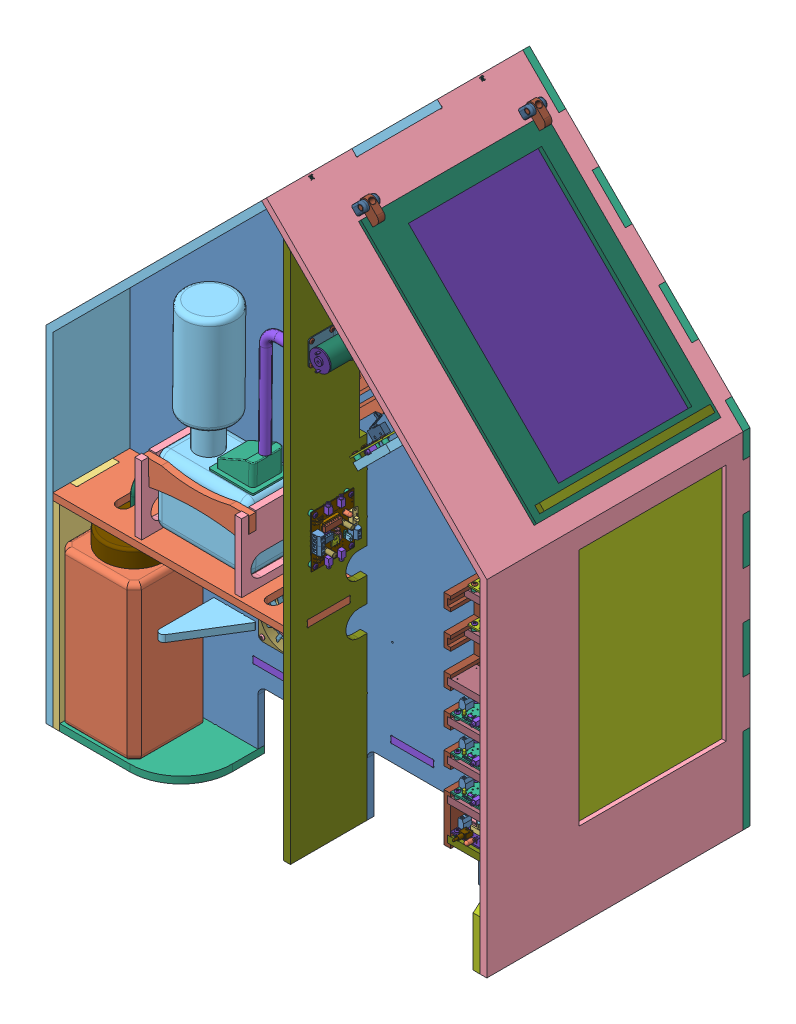
SolidWorks assembly Serre Toutes Options, configuration OLED. Lengths in mm. (continued)
Mates (geometry in assembly coordinates): (continued)
- Coïncidente51: coincident aligned: plane of FONDINTERIEUR-1 through (-297.9367 -225.0262 -4) normal (0 0 -1); plane of VIS TORCX TF 3 X 19-3 through (-31.2492 -313.1905 -4) normal (0 0 -1)
- Coïncidente52: coincident anti-aligned: axis of FONDINTERIEUR-1 through (-30.876 -274.5499 -4) axis (0 0 1); axis of VIS TORCX TF 3 X 19-4 through (-30.876 -274.5499 12.4885) axis (0 0 -1)
- Coïncidente53: coincident aligned: plane of FONDINTERIEUR-1 through (-297.9367 -225.0262 -4) normal (0 0 -1); plane of VIS TORCX TF 3 X 19-4 through (-31.2492 -271.7749 -4) normal (0 0 -1)
- Coïncidente54: coincident anti-aligned: axis of FONDINTERIEUR-1 through (-169.876 -89.9656 -4) axis (0 0 1); axis of VIS TORCX TF 3 X 19-5 through (-169.876 -89.9656 12.4885) axis (0 0 -1)
- Coïncidente55: coincident aligned: plane of FONDINTERIEUR-1 through (-297.9367 -225.0262 -4) normal (0 0 -1); plane of VIS TORCX TF 3 X 19-5 through (-170.2492 -87.1905 -4) normal (0 0 -1)
- Coïncidente56: coincident anti-aligned: axis of FONDINTERIEUR-1 through (-30.876 -27.0369 -4) axis (0 0 1); axis of VIS TORCX TF 3 X 19-6 through (-30.876 -27.0369 12.4885) axis (0 0 -1)
- Coïncidente57: coincident aligned: plane of FONDINTERIEUR-1 through (-297.9367 -225.0262 -4) normal (0 0 -1); plane of VIS TORCX TF 3 X 19-6 through (-31.2492 -24.2619 -4) normal (0 0 -1)
- Coïncidente58: coincident anti-aligned: axis of FONDINTERIEUR-1 through (-30.876 278.5344 -4) axis (0 0 1); axis of VIS TORCX TF 3 X 19-7 through (-30.876 278.5344 12.4885) axis (0 0 -1)
- Coïncidente59: coincident aligned: plane of FONDINTERIEUR-1 through (-297.9367 -225.0262 -4) normal (0 0 -1); plane of VIS TORCX TF 3 X 19-7 through (-31.2492 281.3095 -4) normal (0 0 -1)
- Coïncidente60: coincident anti-aligned: plane of FONDINTERIEUR-1 through (-296.876 -226.0869 4) normal (-1 0 0); plane of Coté gauche serre-1 through (-296.876 -275.0426 -2.9402) normal (1 0 0)
- Coïncidente61: coincident anti-aligned: plane of FONDINTERIEUR-1 through (-298.9973 -273.9656 4) normal (0 1 0); plane of Coté gauche serre-1 through (-296.876 -273.9656 1.8944) normal (0 -1 0)
- Coïncidente62: coincident anti-aligned: plane of FONDINTERIEUR-1 through (-297.9367 -225.0262 -4) normal (0 0 -1); plane of Coté gauche serre-1 through (-296.876 -323.9656 -4) normal (0 0 1)
- Coïncidente63: coincident anti-aligned: plane of FONDINTERIEUR-1 through (-154.876 -315.9656 -4) normal (0 -1 0); plane of suportbloceau-1 through (-297.9367 -315.9656 75.0607) normal (0 1 0)
- Coïncidente64: coincident anti-aligned: plane of FONDINTERIEUR-1 through (-204.876 -318.0869 -4) normal (1 0 0); plane of suportbloceau-1 through (-204.876 -315.9656 -4) normal (-1 0 0)
- Coïncidente65: coincident aligned: plane of FONDINTERIEUR-1 through (-297.9367 -225.0262 -4) normal (0 0 -1); plane of suportbloceau-1 through (-154.876 -315.9656 -4) normal (0 0 -1)
- Coïncidente66: coincident anti-aligned: plane of FONDINTERIEUR-1 through (-95.876 -28.0869 4) normal (1 0 0); plane of Coté support brumisateur-1 through (-95.876 -24.9049 2.9393) normal (-1 0 0)
- Coïncidente67: coincident anti-aligned: plane of FONDINTERIEUR-1 through (-89.9973 -65.9656 4) normal (0 1 0); plane of Coté support brumisateur-1 through (-95.876 -65.9656 -4) normal (0 -1 0)
- Coïncidente68: coincident aligned: plane of FONDINTERIEUR-1 through (-297.9367 -225.0262 -4) normal (0 0 -1); plane of Coté support brumisateur-1 through (-95.876 -25.9656 -4) normal (0 0 -1)
- Coïncidente69: coincident anti-aligned: plane of FONDINTERIEUR-1 through (-212.876 -28.0869 4) normal (1 0 0); plane of Coté support brumisateur-2 through (-212.876 -24.9049 2.9393) normal (-1 0 0)
- Coïncidente70: coincident anti-aligned: plane of FONDINTERIEUR-1 through (-210.7547 -65.9656 4) normal (0 1 0); plane of Coté support brumisateur-2 through (-212.876 -65.9656 -4) normal (0 -1 0)
- Coïncidente71: coincident aligned: plane of FONDINTERIEUR-1 through (-297.9367 -225.0262 -4) normal (0 0 -1); plane of Coté support brumisateur-2 through (-212.876 -25.9656 -4) normal (0 0 -1)
- Coïncidente72: coincident anti-aligned: plane of FONDINTERIEUR-1 through (-189.2547 -195.9656 -4) normal (0 1 0); plane of Renfort bidon-1 through (-192.4367 -195.9656 2.9393) normal (0 -1 0)
- Coïncidente73: coincident anti-aligned: plane of FONDINTERIEUR-1 through (-191.376 -190.0869 -4) normal (1 0 0); plane of Renfort bidon-1 through (-191.376 -187.9656 1.8787) normal (-1 0 0)
- Coïncidente74: coincident aligned: plane of FONDINTERIEUR-1 through (-297.9367 -225.0262 -4) normal (0 0 -1); plane of Renfort bidon-1 through (-191.376 -187.9656 -4) normal (0 0 -1)
- Coïncidente75: coincident aligned: axis of FONDINTERIEUR-1 through (-198.876 -191.9656 4) axis (0 0 -1); axis of VIS TORCX TF 3 X 19-12 through (-198.876 -191.9656 12.4885) axis (0 0 -1)
- Coïncidente76: coincident aligned: plane of FONDINTERIEUR-1 through (-297.9367 -225.0262 -4) normal (0 0 -1); plane of VIS TORCX TF 3 X 19-12 through (-199.9485 -189.3791 -4) normal (0 0 -1)
- Coïncidente77: coincident aligned: axis of FONDINTERIEUR-1 through (-164.4919 -191.9656 4) axis (0 0 -1); axis of VIS TORCX TF 3 X 19-13 through (-164.4919 -191.9656 12.4885) axis (0 0 -1)
- Coïncidente78: coincident aligned: plane of FONDINTERIEUR-1 through (-297.9367 -225.0262 -4) normal (0 0 -1); plane of VIS TORCX TF 3 X 19-13 through (-165.5644 -189.3791 -4) normal (0 0 -1)
- Coïncidente79: coincident aligned: axis of FONDINTERIEUR-1 through (-208.876 -75.9656 4) axis (0 0 -1); axis of VIS TORCX TF 3 X 19-14 through (-208.876 -75.9656 12.4885) axis (0 0 -1)
- Coïncidente80: coincident aligned: plane of FONDINTERIEUR-1 through (-297.9367 -225.0262 -4) normal (0 0 -1); plane of VIS TORCX TF 3 X 19-14 through (-209.9485 -73.3791 -4) normal (0 0 -1)
- Coïncidente81: coincident aligned: axis of FONDINTERIEUR-1 through (-208.876 -16.4656 4) axis (0 0 -1); axis of VIS TORCX TF 3 X 19-15 through (-208.876 -16.4656 12.4885) axis (0 0 -1)
- Coïncidente82: coincident aligned: plane of FONDINTERIEUR-1 through (-297.9367 -225.0262 -4) normal (0 0 -1); plane of VIS TORCX TF 3 X 19-15 through (-209.9485 -13.8791 -4) normal (0 0 -1)
- Coïncidente83: coincident aligned: axis of FONDINTERIEUR-1 through (-91.876 -75.9656 4) axis (0 0 -1); axis of VIS TORCX TF 3 X 19-16 through (-91.876 -75.9656 12.4885) axis (0 0 -1)
- Coïncidente84: coincident aligned: plane of FONDINTERIEUR-1 through (-297.9367 -225.0262 -4) normal (0 0 -1); plane of VIS TORCX TF 3 X 19-16 through (-92.9485 -73.3791 -4) normal (0 0 -1)
- Coïncidente85: coincident aligned: axis of FONDINTERIEUR-1 through (-91.876 -15.9656 4) axis (0 0 -1); axis of VIS TORCX TF 3 X 19-17 through (-91.876 -15.9656 12.4885) axis (0 0 -1)
- Coïncidente86: coincident aligned: plane of FONDINTERIEUR-1 through (-297.9367 -225.0262 -4) normal (0 0 -1); plane of VIS TORCX TF 3 X 19-17 through (-92.9485 -13.3791 -4) normal (0 0 -1)
- Coïncidente87: coincident aligned: axis of Coté gauche serre-1 through (-296.876 -89.9656 48.9996) axis (-1 0 0); axis of VIS TORCX TF 3 X 19-18 through (-288.3875 -89.9656 48.9996) axis (-1 0 0)
- Coïncidente88: coincident aligned: plane of Coté gauche serre-1 through (-304.876 -275.0426 -2.9402) normal (-1 0 0); plane of VIS TORCX TF 3 X 19-18 through (-304.876 -87.1656 48.9996) normal (-1 0 0)
- Coïncidente89: coincident aligned: axis of Coté gauche serre-1 through (-296.876 -248.9656 -0.0009) axis (-1 0 0); axis of VIS TORCX TF 3 X 19-25 through (-288.3875 -248.9656 -0.0009) axis (-1 0 0)
- Coïncidente90: coincident aligned: plane of Coté gauche serre-1 through (-304.876 -275.0426 -2.9402) normal (-1 0 0); plane of VIS TORCX TF 3 X 19-25 through (-304.876 -246.1656 -0.0009) normal (-1 0 0)
- Coïncidente91: coincident aligned: axis of suportbloceau-1 through (-300.876 -315.9656 49) axis (0 -1 0); axis of VIS TORCX TF 3 X 19-26 through (-300.876 -307.477 49) axis (0 -1 0)
- Coïncidente92: coincident aligned: plane of suportbloceau-1 through (-297.9367 -323.9656 75.0607) normal (0 -1 0); plane of VIS TORCX TF 3 X 19-26 through (-299.1327 -323.9656 51.1911) normal (0 -1 0)
- Coïncidente93: coincident aligned: axis of suportbloceau-1 through (-271.876 -315.9656 0) axis (0 -1 0); axis of VIS TORCX TF 3 X 19-29 through (-271.876 -307.477 0) axis (0 -1 0)
- Coïncidente94: coincident aligned: plane of suportbloceau-1 through (-297.9367 -323.9656 75.0607) normal (0 -1 0); plane of VIS TORCX TF 3 X 19-29 through (-270.1327 -323.9656 2.1911) normal (0 -1 0)
- Coïncidente95: coincident aligned: axis of suportbloceau-1 through (-179.876 -315.9656 0) axis (0 -1 0); axis of VIS TORCX TF 3 X 19-30 through (-179.876 -307.477 0) axis (0 -1 0)
- Coïncidente96: coincident aligned: plane of suportbloceau-1 through (-297.9367 -323.9656 75.0607) normal (0 -1 0); plane of VIS TORCX TF 3 X 19-30 through (-178.1327 -323.9656 2.1911) normal (0 -1 0)
- Coïncidente103: coincident anti-aligned: plane of FONDINTERIEUR-1 through (187.124 -226.0869 4) normal (1 0 0); plane of Coté droit serre-1 through (187.124 -275.0262 -2.9393) normal (-1 0 0)
- Coïncidente104: coincident anti-aligned: plane of FONDINTERIEUR-1 through (195.124 -223.9656 4) normal (0 -1 0); plane of Coté droit serre-1 through (195.124 -223.9656 46) normal (0 1 0)
- Coïncidente105: coincident anti-aligned: plane of FONDINTERIEUR-1 through (-297.9367 -225.0262 -4) normal (0 0 -1); plane of Coté droit serre-1 through (195.124 -323.9656 -4) normal (0 0 1)
- Coïncidente114: coincident anti-aligned: axis of Coté droit serre-1 through (195.124 -248.9656 0) axis (-1 0 0); axis of VIS TORCX TF 3 X 19-35 through (178.6355 -248.9656 0) axis (1 0 0)
- Coïncidente115: coincident aligned: plane of Coté droit serre-1 through (195.124 -275.0262 -2.9393) normal (1 0 0); plane of VIS TORCX TF 3 X 19-35 through (195.124 -246.2177 -0.5377) normal (1 0 0)
- Coïncidente116: coincident anti-aligned: plane of FONDINTERIEUR-1 through (48.6689 -231.9656 -4) normal (0 1 0); plane of Poutre fond-1 through (-276.7874 -231.9656 -2.9393) normal (0 -1 0)
- Coïncidente117: coincident anti-aligned: plane of FONDINTERIEUR-1 through (0.7902 -229.8442 -4) normal (1 0 0); plane of Poutre fond-1 through (0.7902 -223.9656 4) normal (-1 0 0)
- Coïncidente118: coincident anti-aligned: plane of FONDINTERIEUR-1 through (-297.9367 -225.0262 -4) normal (0 0 -1); plane of Poutre fond-1 through (-108.4209 -223.9656 -4) normal (0 0 1)
- Coïncidente119: coincident aligned: axis of FONDINTERIEUR-1 through (103.3825 -227.9656 -4) axis (0 0 1); axis of VIS TORCX TF 3 X 19-49 through (103.3825 -227.9656 -12.4885) axis (0 0 1)
- Coïncidente120: coincident aligned: plane of FONDINTERIEUR-1 through (-297.9367 -225.0262 4) normal (0 0 1); plane of VIS TORCX TF 3 X 19-49 through (103.3825 -225.1656 4) normal (0 0 1)
- Coïncidente121: coincident aligned: axis of FONDINTERIEUR-1 through (-54.876 -227.9656 -4) axis (0 0 1); axis of VIS TORCX TF 3 X 19-37 through (-54.876 -227.9656 -12.4885) axis (0 0 1)
- Coïncidente122: coincident aligned: plane of FONDINTERIEUR-1 through (-297.9367 -225.0262 4) normal (0 0 1); plane of VIS TORCX TF 3 X 19-37 through (-54.876 -225.1656 4) normal (0 0 1)
- Coïncidente124: coincident aligned: axis of FONDINTERIEUR-1 through (-213.1345 -227.9656 -4) axis (0 0 1); axis of VIS TORCX TF 3 X 19-36 through (-213.1345 -227.9656 -12.4885) axis (0 0 1)
- Coïncidente125: coincident aligned: plane of FONDINTERIEUR-1 through (-297.9367 -225.0262 4) normal (0 0 1); plane of VIS TORCX TF 3 X 19-36 through (-213.1345 -225.1656 4) normal (0 0 1)
- Coïncidente126: coincident anti-aligned: plane of Poutre fond-1 through (-296.876 -223.9656 -13) normal (0 0 -1); plane of Poutre plateau-1 through (79.7388 -229.6404 -13) normal (0 0 1)
- Coïncidente127: coincident aligned: plane of Coté droit serre-1 through (195.124 -275.0262 -2.9393) normal (1 0 0); plane of Poutre plateau-1 through (195.124 -223.9656 -21) normal (1 0 0)
- Coïncidente128: coincident anti-aligned: plane of Coté droit serre-1 through (195.124 -243.9656 -18.9697) normal (0 1 0); plane of Poutre plateau-1 through (195.124 -243.9656 -21) normal (0 -1 0)
- Coïncidente129: coincident anti-aligned: plane of Coté droit serre-1 through (195.124 -291.8442 -198) normal (0 0 -1); plane of façadeporteplateau-1 through (188.1847 -295.0262 -198) normal (0 0 1)
- Coïncidente130: coincident aligned: plane of Coté droit serre-1 through (195.124 -275.0262 -2.9393) normal (1 0 0); plane of façadeporteplateau-1 through (195.124 -253.9656 -198) normal (1 0 0)
- Coïncidente131: coincident aligned: plane of Coté droit serre-1 through (195.124 -223.9656 -21.091) normal (0 1 0); plane of façadeporteplateau-1 through (-296.876 -223.9656 -198) normal (0 1 0)
- Coïncidente132: coincident anti-aligned: axis of Coté droit serre-1 through (195.124 -238.9656 -202) axis (-1 0 0); axis of VIS TORCX TF 3 X 19-40 through (178.6355 -238.9656 -202) axis (1 0 0)
- Coïncidente133: coincident aligned: plane of Coté droit serre-1 through (195.124 -275.0262 -2.9393) normal (1 0 0); plane of VIS TORCX TF 3 X 19-40 through (195.124 -236.1656 -202) normal (1 0 0)
- Coïncidente134: coincident anti-aligned: axis of Coté droit serre-1 through (195.124 -308.9656 -202) axis (-1 0 0); axis of VIS TORCX TF 3 X 19-39 through (178.6355 -308.9656 -202) axis (1 0 0)
- Coïncidente135: coincident aligned: plane of Coté droit serre-1 through (195.124 -275.0262 -2.9393) normal (1 0 0); plane of VIS TORCX TF 3 X 19-39 through (195.124 -306.1656 -202) normal (1 0 0)
- Coïncidente136: coincident aligned: axis of façadeporteplateau-1 through (191.124 -273.9656 -198) axis (0 0 -1); axis of VIS TORCX TF 3 X 19-38 through (191.124 -273.9656 -189.5115) axis (0 0 -1)
- Coïncidente137: coincident aligned: plane of façadeporteplateau-1 through (188.1847 -295.0262 -206) normal (0 0 -1); plane of VIS TORCX TF 3 X 19-38 through (190.0515 -271.3791 -206) normal (0 0 -1)
- Coïncidente138: coincident aligned: axis of façadeporteplateau-1 through (-300.876 -273.9656 -198) axis (0 0 -1); axis of VIS TORCX TF 3 X 19-43 through (-300.876 -273.9656 -189.5115) axis (0 0 -1)
- Coïncidente139: coincident aligned: plane of façadeporteplateau-1 through (188.1847 -295.0262 -206) normal (0 0 -1); plane of VIS TORCX TF 3 X 19-43 through (-301.9485 -271.3791 -206) normal (0 0 -1)
- Coïncidente140: coincident aligned: axis of Coté gauche serre-1 through (-296.876 -238.9737 -202) axis (-1 0 0); axis of VIS TORCX TF 3 X 19-44 through (-288.3875 -238.9737 -202) axis (-1 0 0)
- Coïncidente141: coincident aligned: plane of Coté gauche serre-1 through (-304.876 -275.0426 -2.9402) normal (-1 0 0); plane of VIS TORCX TF 3 X 19-44 through (-304.876 -236.1737 -202) normal (-1 0 0)
- Coïncidente142: coincident aligned: axis of Coté gauche serre-1 through (-296.876 -308.9656 -202) axis (-1 0 0); axis of VIS TORCX TF 3 X 19-45 through (-288.3875 -308.9656 -202) axis (-1 0 0)
- Coïncidente143: coincident aligned: plane of Coté gauche serre-1 through (-304.876 -275.0426 -2.9402) normal (-1 0 0); plane of VIS TORCX TF 3 X 19-45 through (-304.876 -306.1656 -202) normal (-1 0 0)
- Coïncidente144: coincident anti-aligned: plane of FONDINTERIEUR-1 through (112.8547 -40.3939 -4) normal (1 0 0); plane of Sous ensemble Rack module Toutes Options-1/rack coté gauche-1 through (112.8547 -36.9223 2.9393) normal (-1 0 0)
- Coïncidente145: coincident anti-aligned: plane of FONDINTERIEUR-1 through (176.9761 -37.9656 -4) normal (0 -1 0); plane of Sous ensemble Rack module Toutes Options-1/rack coté droit-1 through (182.8547 -37.9656 1.8787) normal (0 1 0)
- Coïncidente146: coincident aligned: plane of FONDINTERIEUR-1 through (-297.9367 -225.0262 -4) normal (0 0 -1); plane of Sous ensemble Rack module Toutes Options-1/rack coté droit-1 through (182.8547 -37.9656 -4) normal (0 0 -1)
- Coïncidente147: coincident aligned: axis of FONDINTERIEUR-1 through (178.8547 -145.9656 4) axis (0 0 -1); axis of VIS TORCX TF 3 X 19-50 through (178.8547 -145.9656 12.4885) axis (0 0 -1)
- Coïncidente148: coincident aligned: plane of FONDINTERIEUR-1 through (-297.9367 -225.0262 -4) normal (0 0 -1); plane of VIS TORCX TF 3 X 19-50 through (177.7822 -143.3791 -4) normal (0 0 -1)
- Coïncidente149: coincident aligned: axis of FONDINTERIEUR-1 through (116.8547 -145.9656 4) axis (0 0 -1); axis of VIS TORCX TF 3 X 19-51 through (116.8547 -145.9656 12.4885) axis (0 0 -1)
- Coïncidente150: coincident aligned: plane of FONDINTERIEUR-1 through (-297.9367 -225.0262 -4) normal (0 0 -1); plane of VIS TORCX TF 3 X 19-51 through (115.7822 -143.3791 -4) normal (0 0 -1)
- Coïncidente151: coincident anti-aligned: axis of FONDINTERIEUR-1 through (178.8547 -7.9656 -4) axis (0 0 1); axis of VIS TORCX TF 3 X 19-52 through (178.8547 -7.9656 12.4885) axis (0 0 -1)
- Coïncidente152: coincident aligned: plane of FONDINTERIEUR-1 through (-297.9367 -225.0262 -4) normal (0 0 -1); plane of VIS TORCX TF 3 X 19-52 through (177.7822 -5.3791 -4) normal (0 0 -1)
- Coïncidente153: coincident anti-aligned: axis of FONDINTERIEUR-1 through (116.8547 -7.9656 -4) axis (0 0 1); axis of VIS TORCX TF 3 X 19-53 through (116.8547 -7.9656 12.4885) axis (0 0 -1)
- Coïncidente154: coincident aligned: plane of FONDINTERIEUR-1 through (-297.9367 -225.0262 -4) normal (0 0 -1); plane of VIS TORCX TF 3 X 19-53 through (115.7822 -5.3791 -4) normal (0 0 -1)
- Coïncidente163: coincident aligned: axis of FONDINTERIEUR-1 through (-255.126 -66.1655 -4) axis (0 0 1); axis of Sous ensemble Arrosage-1/Tuyau gouteur-1 through (-255.126 -66.1655 -11.25) axis (0 0 1)
- Coïncidente164: coincident anti-aligned: plane of suportbloceau-1 through (-297.9367 -315.9656 75.0607) normal (0 1 0); plane of Sous ensemble Arrosage-1/Reservoir 1,25L-1 through (-272.5 -315.9655 45.1435) normal (0 -1 0)
- Coïncidente168: coincident anti-aligned: plane of FONDINTERIEUR-1 through (-297.9367 -225.0262 4) normal (0 0 1); plane of Sous ensemble Arrosage-1/Reservoir 1,25L-1 through (-299.876 -315.9655 4) normal (0 0 -1)
- Coïncidente178: coincident anti-aligned: axis of FONDINTERIEUR-1 through (152.3558 6.7126 -4) axis (0 0 1); axis of fondcuivré-1 through (152.3558 6.7126 -4) axis (0 0 -1)
- Coïncidente179: coincident anti-aligned: plane of FONDINTERIEUR-1 through (-297.9367 -225.0262 -4) normal (0 0 -1); plane of fondcuivré-1 through (-208.3657 -251.1382 -4) normal (0 0 1)
- Parallèle5: parallel anti-aligned: line of FONDINTERIEUR-1 through (-62.876 322.2771 -4) axis (1 0 0); line of fondcuivré-1 through (-29.876 291.0344 -5) axis (-1 0 0)
- Coïncidente180: coincident anti-aligned: plane of façadeporteplateau-1 through (188.1847 -295.0262 -206) normal (0 0 -1); plane of Capot complet-1/Capotfaçade-1 through (-305.9367 -222.9049 -206) normal (0 0 1)
- Coïncidente181: coincident aligned: plane of façadeporteplateau-1 through (-296.876 -323.9656 -198) normal (0 -1 0); plane of Capot complet-1/Capotfaçade-1 through (-312.876 -323.9656 -206) normal (0 -1 0)
- Coïncidente182: coincident anti-aligned: line of Coté droit serre-1 through (195.124 -323.9656 -4) axis (0 0 -1); line of Capot complet-1/Capot coté droit-1 through (195.124 -323.9656 -206) axis (0 0 1)
- Coïncidente185: coincident anti-aligned: plane of Capot complet-1/Capotfaçade-1 through (-305.9367 -222.9049 -214) normal (0 0 -1); plane of Cache Oled-2 through (-241.7989 -284.4707 -214) normal (0 0 1)
- Coïncidente186: coincident aligned: line of guillotine-1 through (-87.876 -25.9656 81.5) axis (0 0 -1); line of Coté support brumisateur-1 through (-87.876 -25.9656 82) axis (0 0 -1)
- Coïncidente187: coincident aligned: plane of Coté support brumisateur-1 through (-87.876 -24.9049 2.9393) normal (1 0 0); plane of guillotine-1 through (-87.876 -7.5675 81.5) normal (1 0 0)
- Coïncidente189: coincident anti-aligned: plane of Coté support brumisateur-1 through (-95.876 -25.9656 73.5) normal (0 0 1); plane of guillotine-1 through (-150.376 149.9325 73.5) normal (0 0 -1)
- Coïncidente191: coincident anti-aligned: axis of façadeporteplateau-1 through (-160.876 -263.4656 -202) axis (0 0 1); axis of Entretoise CI-3 through (-160.876 -263.4656 -193.9) axis (0 0 -1)
- Coïncidente192: coincident aligned: plane of façadeporteplateau-1 through (188.1847 -295.0262 -198) normal (0 0 1); circle of Entretoise CI-3
- Coïncidente193: coincident anti-aligned: axis of façadeporteplateau-1 through (-160.876 -285.4656 -202) axis (0 0 1); axis of Entretoise CI-4 through (-160.876 -285.4656 -193.9) axis (0 0 -1)
- Coïncidente194: coincident aligned: plane of façadeporteplateau-1 through (188.1847 -295.0262 -198) normal (0 0 1); circle of Entretoise CI-4
- Coïncidente195: coincident anti-aligned: axis of façadeporteplateau-1 through (-114.876 -263.4656 -202) axis (0 0 1); axis of Entretoise CI-5 through (-114.876 -263.4656 -193.9) axis (0 0 -1)
- Coïncidente196: coincident aligned: plane of façadeporteplateau-1 through (188.1847 -295.0262 -198) normal (0 0 1); circle of Entretoise CI-5
- Coïncidente197: coincident anti-aligned: axis of façadeporteplateau-1 through (-114.876 -285.4656 -202) axis (0 0 1); axis of Entretoise CI-6 through (-114.876 -285.4656 -193.9) axis (0 0 -1)
- Coïncidente198: coincident aligned: plane of façadeporteplateau-1 through (188.1847 -295.0262 -198) normal (0 0 1); circle of Entretoise CI-6
- Coïncidente199: coincident anti-aligned: axis of façadeporteplateau-1 through (-101.8754 -258.9657 -202) axis (0 0 1); axis of Entretoise CI-7 through (-101.8754 -258.9657 -193.9) axis (0 0 -1)
- Coïncidente200: coincident aligned: plane of façadeporteplateau-1 through (188.1847 -295.0262 -198) normal (0 0 1); circle of Entretoise CI-7
- Coïncidente201: coincident anti-aligned: axis of façadeporteplateau-1 through (-101.8754 -304.9651 -202) axis (0 0 1); axis of Entretoise CI-8 through (-101.8754 -304.9651 -193.9) axis (0 0 -1)
- Coïncidente202: coincident aligned: plane of façadeporteplateau-1 through (188.1847 -295.0262 -198) normal (0 0 1); circle of Entretoise CI-8
- Coïncidente203: coincident anti-aligned: axis of façadeporteplateau-1 through (-79.8765 -258.9657 -202) axis (0 0 1); axis of Entretoise CI-9 through (-79.8765 -258.9657 -193.9) axis (0 0 -1)
- Coïncidente204: coincident aligned: plane of façadeporteplateau-1 through (188.1847 -295.0262 -198) normal (0 0 1); circle of Entretoise CI-9
- Coïncidente205: coincident anti-aligned: axis of façadeporteplateau-1 through (-79.8765 -304.9651 -202) axis (0 0 1); axis of Entretoise CI-10 through (-79.8765 -304.9651 -193.9) axis (0 0 -1)
- Coïncidente206: coincident aligned: plane of façadeporteplateau-1 through (188.1847 -295.0262 -198) normal (0 0 1); circle of Entretoise CI-10
- Coïncidente215: coincident aligned: axis of façadeporteplateau-1 through (-160.876 -263.4656 -202) axis (0 0 1); axis of Module Bouton poussoir K-AP-MBP-1/CI-AP-MLBP avec jack-1/CI BP et DEL-1 through (-160.876 -263.4656 -193.9) axis (0 0 1)
- Coïncidente216: coincident aligned: axis of façadeporteplateau-1 through (-114.876 -263.4656 -202) axis (0 0 1); axis of Module Bouton poussoir K-AP-MBP-1/CI-AP-MLBP avec jack-1/CI BP et DEL-1 through (-114.8766 -263.4656 -193.9) axis (0 0 1)
- Coïncidente217: coincident anti-aligned: plane of Module Bouton poussoir K-AP-MBP-1/CI-AP-MLBP avec jack-1/CI BP et DEL-1 through (-110.8765 -289.465 -193.9) normal (0 0 -1); plane of Entretoise CI-3 through (-160.876 -263.4656 -193.9) normal (0 0 1)
- Coïncidente218: coincident anti-aligned: axis of façadeporteplateau-1 through (-101.8754 -258.9657 -202) axis (0 0 1); axis of K-AP-MOLED-1/CI AP-EIR avec embase-1/CI AP-EIR-1 through (-101.8754 -258.9657 -192.3) axis (0 0 -1)
- Coïncidente219: coincident anti-aligned: axis of façadeporteplateau-1 through (-101.8754 -304.9651 -202) axis (0 0 1); axis of K-AP-MOLED-1/CI AP-EIR avec embase-1/CI AP-EIR-1 through (-101.8754 -304.9651 -192.3) axis (0 0 -1)
- Coïncidente220: coincident anti-aligned: plane of K-AP-MOLED-1/CI AP-EIR avec embase-1/CI AP-EIR-1 through (-75.876 -254.9652 -193.9) normal (0 0 -1); plane of Entretoise CI-8 through (-101.8754 -304.9651 -193.9) normal (0 0 1)
- Distance2: distance = 0.5 mm anti-aligned: plane of façadeporteplateau-1 through (-271.9769 -257.9656 -208) normal (0 -1 0); plane of OLED 4 lignes-1/OLED Ecran-1 through (-180.376 -258.4656 -204.3) normal (0 1 0)
- Distance3: distance = 0.5 mm anti-aligned: plane of façadeporteplateau-1 through (-179.876 -260.8647 -208) normal (-1 0 0); plane of OLED 4 lignes-1/OLED Ecran-1 through (-180.376 -258.4656 -204.3) normal (1 0 0)
- Coïncidente229: coincident aligned: plane of façadeporteplateau-1 through (188.1847 -295.0262 -198) normal (0 0 1); plane of OLED 4 lignes-1/OLED Ecran-1 through (-241.2768 -276.4561 -198) normal (0 0 1)
- Coïncidente230: coincident aligned: axis of Module Bouton poussoir K-AP-MBP-1/CI-AP-MLBP avec jack-1/CI BP et DEL-1 through (-160.876 -263.4656 -193.9) axis (0 0 1); axis of VIs TC 3 x 9-1 through (-160.876 -263.4656 -198.8) axis (0 0 1)
- Coïncidente231: coincident aligned: axis of Module Bouton poussoir K-AP-MBP-1/CI-AP-MLBP avec jack-1/CI BP et DEL-1 through (-160.876 -285.4645 -193.9) axis (0 0 1); axis of VIs TC 3 x 9-2 through (-160.876 -285.4645 -198.8) axis (0 0 1)
- Coïncidente232: coincident aligned: axis of Module Bouton poussoir K-AP-MBP-1/CI-AP-MLBP avec jack-1/CI BP et DEL-1 through (-114.8766 -263.4656 -193.9) axis (0 0 1); axis of VIs TC 3 x 9-3 through (-114.876 -263.4656 -198.8) axis (0 0 1)
- Coïncidente233: coincident aligned: axis of Module Bouton poussoir K-AP-MBP-1/CI-AP-MLBP avec jack-1/CI BP et DEL-1 through (-114.8766 -285.4645 -193.9) axis (0 0 1); axis of VIs TC 3 x 9-4 through (-114.8766 -285.4645 -198.8) axis (0 0 1)
- Coïncidente234: coincident anti-aligned: axis of K-AP-MOLED-1/CI AP-EIR avec embase-1/CI AP-EIR-1 through (-101.8754 -258.9657 -192.3) axis (0 0 -1); axis of VIs TC 3 x 9-5 through (-101.8754 -258.9657 -198.8) axis (0 0 1)
- Coïncidente235: coincident anti-aligned: axis of K-AP-MOLED-1/CI AP-EIR avec embase-1/CI AP-EIR-1 through (-79.8765 -258.9657 -192.3) axis (0 0 -1); axis of VIs TC 3 x 9-6 through (-79.8765 -258.9657 -198.8) axis (0 0 1)
- Coïncidente236: coincident anti-aligned: axis of K-AP-MOLED-1/CI AP-EIR avec embase-1/CI AP-EIR-1 through (-101.8754 -304.9651 -192.3) axis (0 0 -1); axis of VIs TC 3 x 9-7 through (-101.8754 -304.9651 -198.8) axis (0 0 1)
- Coïncidente237: coincident anti-aligned: axis of K-AP-MOLED-1/CI AP-EIR avec embase-1/CI AP-EIR-1 through (-79.8765 -304.9651 -192.3) axis (0 0 -1); axis of VIs TC 3 x 9-8 through (-79.8765 -304.9651 -198.8) axis (0 0 1)
- Coïncidente238: coincident anti-aligned: plane of K-AP-MOLED-1/CI AP-EIR avec embase-1/CI AP-EIR-1 through (-75.876 -254.9652 -192.3) normal (0 0 1); plane of VIs TC 3 x 9-8 through (-79.8765 -304.9651 -192.3) normal (0 0 -1)
- Coïncidente239: coincident anti-aligned: plane of K-AP-MOLED-1/CI AP-EIR avec embase-1/CI AP-EIR-1 through (-75.876 -254.9652 -192.3) normal (0 0 1); plane of VIs TC 3 x 9-7 through (-101.8754 -304.9651 -192.3) normal (0 0 -1)
- Coïncidente240: coincident anti-aligned: plane of K-AP-MOLED-1/CI AP-EIR avec embase-1/CI AP-EIR-1 through (-75.876 -254.9652 -192.3) normal (0 0 1); plane of VIs TC 3 x 9-6 through (-79.8765 -258.9657 -192.3) normal (0 0 -1)
- Coïncidente241: coincident anti-aligned: plane of K-AP-MOLED-1/CI AP-EIR avec embase-1/CI AP-EIR-1 through (-75.876 -254.9652 -192.3) normal (0 0 1); plane of VIs TC 3 x 9-5 through (-101.8754 -258.9657 -192.3) normal (0 0 -1)
- Coïncidente242: coincident anti-aligned: plane of Module Bouton poussoir K-AP-MBP-1/CI-AP-MLBP avec jack-1/CI BP et DEL-1 through (-110.8765 -289.465 -192.3) normal (0 0 1); plane of VIs TC 3 x 9-3 through (-114.876 -263.4656 -192.3) normal (0 0 -1)
- Coïncidente243: coincident anti-aligned: plane of Module Bouton poussoir K-AP-MBP-1/CI-AP-MLBP avec jack-1/CI BP et DEL-1 through (-110.8765 -289.465 -192.3) normal (0 0 1); plane of VIs TC 3 x 9-4 through (-114.8766 -285.4645 -192.3) normal (0 0 -1)
- Coïncidente244: coincident anti-aligned: plane of Module Bouton poussoir K-AP-MBP-1/CI-AP-MLBP avec jack-1/CI BP et DEL-1 through (-110.8765 -289.465 -192.3) normal (0 0 1); plane of VIs TC 3 x 9-1 through (-160.876 -263.4656 -192.3) normal (0 0 -1)
- Coïncidente245: coincident anti-aligned: plane of Module Bouton poussoir K-AP-MBP-1/CI-AP-MLBP avec jack-1/CI BP et DEL-1 through (-110.8765 -289.465 -192.3) normal (0 0 1); plane of VIs TC 3 x 9-2 through (-160.876 -285.4645 -192.3) normal (0 0 -1)
- Coïncidente246: coincident anti-aligned: axis of OLED 4 lignes-1/OLED Ecran-1 through (-273.876 -246.9656 -199.55) axis (0 0 1); axis of VIs TC 3 x 6.5-1 through (-273.876 -246.9656 -198) axis (0 0 -1)
- Coïncidente247: coincident anti-aligned: axis of OLED 4 lignes-1/OLED Ecran-1 through (-180.876 -301.9656 -199.55) axis (0 0 1); axis of VIs TC 3 x 6.5-2 through (-180.876 -301.9656 -198) axis (0 0 -1)
- Coïncidente248: coincident anti-aligned: axis of OLED 4 lignes-1/OLED Ecran-1 through (-273.876 -301.9656 -199.55) axis (0 0 1); axis of VIs TC 3 x 6.5-3 through (-273.876 -301.9656 -198) axis (0 0 -1)
- Coïncidente249: coincident anti-aligned: plane of OLED 4 lignes-1/OLED Ecran-1 through (-241.2768 -276.4561 -198) normal (0 0 1); plane of VIs TC 3 x 6.5-1 through (-273.876 -246.9656 -198) normal (0 0 -1)
- Coïncidente250: coincident anti-aligned: plane of OLED 4 lignes-1/OLED Ecran-1 through (-241.2768 -276.4561 -198) normal (0 0 1); plane of VIs TC 3 x 6.5-3 through (-273.876 -301.9656 -198) normal (0 0 -1)
- Coïncidente251: coincident anti-aligned: plane of OLED 4 lignes-1/OLED Ecran-1 through (-241.2768 -276.4561 -198) normal (0 0 1); plane of VIs TC 3 x 6.5-2 through (-180.876 -301.9656 -198) normal (0 0 -1)
- Coïncidente252: coincident anti-aligned: plane of Coté gauche serre-1 through (-300.876 -234.7377 -200.7951) normal (1 0 0); plane of Plateau chauffant-1/Plateau chauffant desssous-1 through (-300.876 -235.9656 -202) normal (-1 0 0)
- Coïncidente253: coincident anti-aligned: plane of façadeporteplateau-1 through (102.5126 -276.3164 -202) normal (0 0 1); plane of Plateau chauffant-1/Plateau chauffant desssous-1 through (191.124 -235.9656 -202) normal (0 0 -1)
- Coïncidente254: coincident anti-aligned: plane of façadeporteplateau-1 through (-311.8157 -235.9656 -202) normal (0 1 0); plane of Plateau chauffant-1/Plateau chauffant desssous-1 through (121.0164 -235.9656 -41.3241) normal (0 -1 0)
- Coïncidente255: coincident aligned: axis of FONDINTERIEUR-1 through (-54.876 305.2771 -4) axis (0 0 1); axis of Sous ensemble Brumisateur complet-1/picobrumisateurbis-1 through (-54.876 305.2771 -5.9737) axis (0 0 1)
- Coïncidente257: coincident: axis of VIS TORCX TF 3 X 19-15 through (-208.876 -16.4656 12.4885) axis (0 0 1); plane of Sous ensemble Brumisateur complet-1/volumebrumi-1 through (-208.7623 -4.247 72) normal (-0.999957 0.009304 0)
- Coïncidente258: coincident anti-aligned: plane of FONDINTERIEUR-1 through (-297.9367 -225.0262 -4) normal (0 0 -1); plane of Sous ensemble Brumisateur complet-1/picobrumisateurbis-1 through (-46.8763 305.2026 -4) normal (0 0 1)
